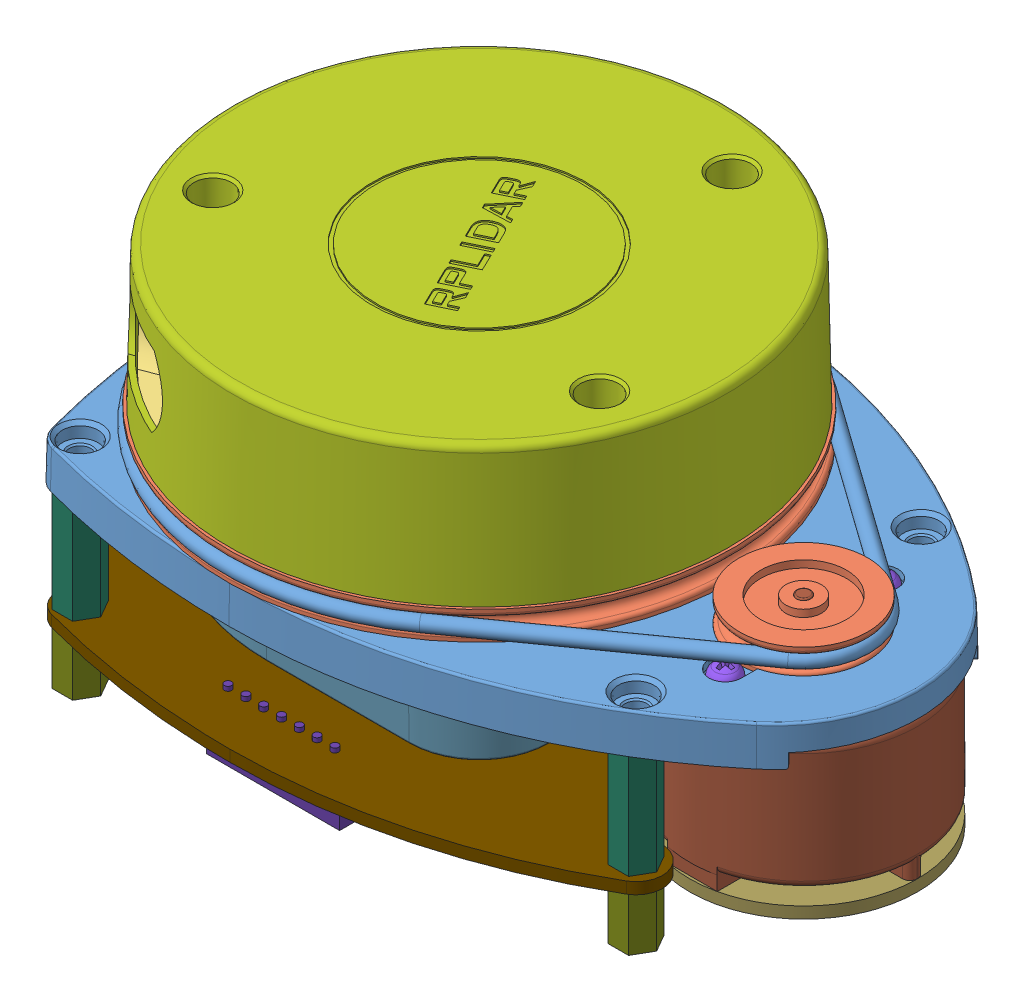
SolidWorks assembly RP-lidar-A1, configuration Default. Lengths in mm.
Overall size (125.66 53.5 112.5).
31 component instances, 20 part files, 0 mates.
Components (placement in the parent):
- RP-lidar-A1.igs-1: RP-lidar-A1.igs [Default] at origin size (125.66 53.5 112.5)
  - base.igs-1: base.igs [Default] at (-90.5533 748.2923 132.9176) size (107.5 12.7 70.46)
  - head-base.igs-1: head-base.igs [Default] at (-90.5533 751.2923 132.9176) x (0.900173 0 -0.435532) z (0.435532 0 0.900173) size (78.94 21.4 82.8)
  - detector-mount.igs-1: detector-mount.igs [Default] at (-90.4238 754.2923 132.7756) x (-0.437519 0 -0.899209) z (0.899209 0 -0.437519) size (22.2 19.69 24.64)
  - detector.igs-1: detector.igs [Default] at (-93.3269 763.2923 153.0936) x (-0.088661 0.979252 -0.182219) z (-0.899209 0 0.437519) size (14.42 15.28 11.5)
  - laser.igs-1: laser.igs [Default] at (-96.1268 764.2923 107.8262) x (0.382786 0.720375 0.578389) z (-0.833913 0 0.551896) size (6.5 8.25 21.2)
  - laser-mount.igs-1: laser-mount.igs [Default] at (-90.5533 755.2923 132.9176) x (-0.430466 0 -0.902607) z (0.902607 0 -0.430466) size (15.26 18.5 21.53)
  - head.igs-1: head.igs [Default] at (-90.5533 773.1923 132.9176) x (0.435532 0 0.900173) z (0.900173 0 -0.435532) size (84.91 19.5 78.26)
  - Woodscrews_GB_TYPE136 M2X6-N.igs-1: Woodscrews_GB_TYPE136 M2X6-N.igs [Default] at (-64.2029 766.7923 142.3864) x (0 -1 0) z (-0.876166 0 -0.482009) size (7.56 3.91 3.91)
  - Woodscrews_GB_TYPE136 M2X6-N.igs-2: Woodscrews_GB_TYPE136 M2X6-N.igs [Default] at (-81.6242 766.7923 106.3795) x (0 -1 0) z (-0.876166 0 -0.482009) size (7.56 3.91 3.91)
  - Woodscrews_GB_TYPE136 M2X6-N.igs-3: Woodscrews_GB_TYPE136 M2X6-N.igs [Default] at (-115.7581 766.7923 145.1125) x (0 -1 0) z (-0.922446 0 -0.386125) size (7.56 3.91 3.91)
  - Woodscrews_GB_TYPE136 M2X6-N.igs-4: Woodscrews_GB_TYPE136 M2X6-N.igs [Default] at (-45.0533 750.5923 121.9176) x (0 -1 0) z (0.032922 0 0.999458) size (7.56 3.91 3.91)
  - Woodscrews_GB_TYPE136 M2X6-N.igs-5: Woodscrews_GB_TYPE136 M2X6-N.igs [Default] at (-45.0533 750.5923 143.9176) x (0 -1 0) z (0.032922 0 0.999458) size (7.56 3.91 3.91)
  - motherboard.igs-1: motherboard.igs [Default] at (-90.5533 738.2923 132.9176) size (55.5 1 57)
  - connector-1_25-3pin.igs-1: connector-1_25-3pin.igs [Default] at (-57.5533 723.4923 132.5551) x (0 0 1) z (0 -1 0) size (8.9 5.2 3.4)
  - motor.igs-1: motor.igs [Default] at (-45.0533 728.7923 132.9176) x (0 0 1) z (-1 0 0) size (32.79 30.2 32.01)
  - motor-board.igs-1: motor-board.igs [Default] at (-45.0533 725.1923 132.9176) x (0.420142 0 0.907458) z (-0.907458 0 0.420142) size (32 1.6 32)
  - connector-1_25-4pin.igs-1: connector-1_25-4pin.igs [Default] at (-68.3533 736.4423 132.7926) x (0 0 1) z (1 0 0) size (10.15 4.2 4.7)
  - bottom-lid.igs-1: bottom-lid.igs [Default] at (-90.5533 737.2923 132.9176) size (61.38 11.06 61.97)
  - stand_15x2.igs-1: stand_15x2.igs [Default] at (-118.5533 729.2923 160.9176) size (5.77 15 5)
  - stand_15x2.igs-2: stand_15x2.igs [Default] at (-48.5533 729.2923 152.9176) size (5.77 15 5)
  - stand_15x2.igs-3: stand_15x2.igs [Default] at (-48.5533 729.2923 112.9176) size (5.77 15 5)
  - stand_15x2.igs-4: stand_15x2.igs [Default] at (-118.5533 729.2923 104.9176) size (5.77 15 5)
  - stand-8x2.igs-1: stand-8x2.igs [Default] at (-48.5533 727.6923 152.9176) x (1 0 0) z (0 0 -1) size (5.77 8 5)
  - stand-8x2.igs-2: stand-8x2.igs [Default] at (-118.5533 727.6923 160.9176) x (1 0 0) z (0 0 -1) size (5.77 8 5)
  - stand-8x2.igs-3: stand-8x2.igs [Default] at (-118.5533 727.6923 104.9176) x (1 0 0) z (0 0 -1) size (5.77 8 5)
  - stand-8x2.igs-4: stand-8x2.igs [Default] at (-48.5533 727.6923 112.9176) x (1 0 0) z (0 0 -1) size (5.77 8 5)
  - connector-7pin-2_5.igs-1: connector-7pin-2_5.igs [Default] at (-90.5533 727.6923 160.0176) x (0 -1 0) z (1 0 0) size (8.2 5 20)
  - devboard.igs-1: devboard.igs [Default] at (-90.5533 729.2923 132.9176) x (1 0 0) z (0 0 -1) size (85.1 7.64 70)
  - rubber.igs-1: rubber.igs [Default] at (-90.5533 751.4783 132.9176) x (1 0 0) z (0 -1 0) size (103.16 95.72 2.15)
  - wheel.igs-1: wheel.igs [Default] at (-45.0533 749.2923 132.9176) x (-0.124101 0 -0.99227) z (0.99227 0 -0.124101) size (18 5.5 18)
